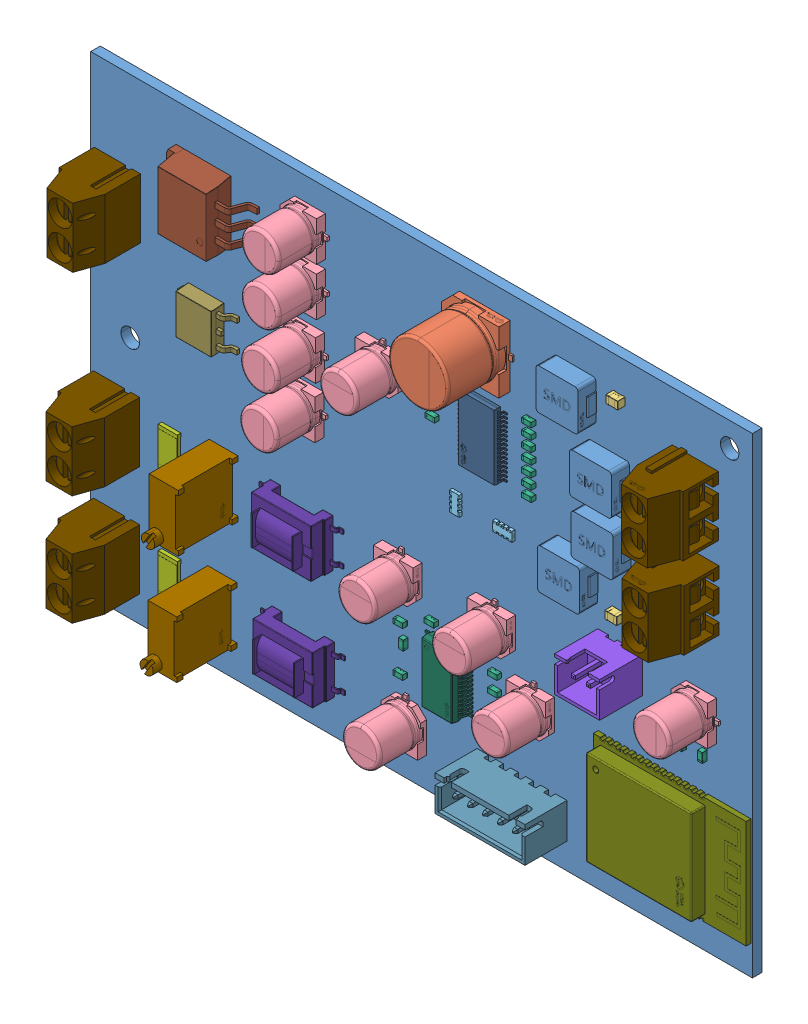
SolidWorks assembly 3D_I2SInputAmp_1_2024-11-02, configuration 默认. Lengths in mm.
Overall size (110.46 78.71 15.8).
191 component instances, 19 part files, 0 mates.
Components (placement in the parent):
- 3D_I2SInputAmp_1_2024-11-02.step-1: 3D_I2SInputAmp_1_2024-11-02.step [默认] at origin size (110.46 78.71 15.8)
  - 2uP9-L2.step-1: 2uP9-L2.step [默认] at (86.2332 60.9601 1.6001) size (7.42 6.8 3.05)
    - IND-SMD_L7.3-W6.8.step-1: IND-SMD_L7.3-W6.8.step [默认] at origin size (7.42 6.8 3.05)
      - SOLID.step-1: SOLID.step [默认] at origin size (7.42 6.8 3.05)
  - 2uP9-L3.step-1: 2uP9-L3.step [默认] at (86.4872 52.1971 1.6001) size (7.42 6.8 3.05)
    - IND-SMD_L7.3-W6.8.step-1: IND-SMD_L7.3-W6.8.step [默认] at origin size (7.42 6.8 3.05)
      - SOLID.step-1: SOLID.step [默认] at origin size (7.42 6.8 3.05)
  - 2uP9-L4.step-1: 2uP9-L4.step [默认] at (80.8992 44.4501 1.6001) size (7.42 6.8 3.05)
    - IND-SMD_L7.3-W6.8.step-1: IND-SMD_L7.3-W6.8.step [默认] at origin size (7.42 6.8 3.05)
      - SOLID.step-1: SOLID.step [默认] at origin size (7.42 6.8 3.05)
  - 2uP9-L1.step-1: 2uP9-L1.step [默认] at (80.6452 70.3581 1.6001) size (7.42 6.8 3.05)
    - IND-SMD_L7.3-W6.8.step-1: IND-SMD_L7.3-W6.8.step [默认] at origin size (7.42 6.8 3.05)
      - SOLID.step-1: SOLID.step [默认] at origin size (7.42 6.8 3.05)
  - 2uP9-C111.step-1: 2uP9-C111.step [默认] at (64.6431 69.7231 1.6001) size (11.6 10.3 10.21)
    - CAP-SMD_BD10.0-L10.3-W10.3-LS11.0-FD.step-1: CAP-SMD_BD10.0-L10.3-W10.3-LS11.0-FD.step [默认] at origin size (11.6 10.3 10.21)
      - COMPOUND.step-1: COMPOUND.step [默认] at origin size (11.6 10.3 10.21)
  - 2uP9-C108.step-1: 2uP9-C108.step [默认] at (87.8528 41.5212 1.6001) x (-1 0 0) z (0 0 1) size (2 1.3 1.3)
    - C0805.step-1: C0805.step [默认] at origin size (2 1.3 1.3)
      - SOLID-0.step-1: SOLID-0.step [默认] at origin size (2 1.3 1.3)
  - 2uP9-C109.step-1: 2uP9-C109.step [默认] at (92.4562 48.6411 1.6001) x (0 1 0) z (0 0 1) size (2 1.3 1.3)
    - C0805.step-1: C0805.step [默认] at origin size (2 1.3 1.3)
      - SOLID-0.step-1: SOLID-0.step [默认] at origin size (2 1.3 1.3)
  - 2uP9-C110.step-1: 2uP9-C110.step [默认] at (93.2182 62.7381 1.6001) x (0 -1 0) z (0 0 1) size (2 1.3 1.3)
    - C0805.step-1: C0805.step [默认] at origin size (2 1.3 1.3)
      - SOLID-0.step-1: SOLID-0.step [默认] at origin size (2 1.3 1.3)
  - 2uP9-C107.step-1: 2uP9-C107.step [默认] at (88.0112 72.7711 1.6001) size (2 1.3 1.3)
    - C0805.step-1: C0805.step [默认] at origin size (2 1.3 1.3)
      - SOLID-0.step-1: SOLID-0.step [默认] at origin size (2 1.3 1.3)
  - 2uP9-C93.step-1: 2uP9-C93.step [默认] at (35.6871 71.6281 1.6001) size (7.8 6.6 7.75)
    - CAP-SMD_BD6.3-L6.6-W6.6-FD.step-1: CAP-SMD_BD6.3-L6.6-W6.6-FD.step [默认] at origin size (7.8 6.6 7.75)
      - SOLID-1.step-1: SOLID-1.step [默认] at origin size (7.8 6.6 7.75)
  - 2uP9-C94.step-1: 2uP9-C94.step [默认] at (35.6871 63.6271 1.6001) size (7.8 6.6 7.75)
    - CAP-SMD_BD6.3-L6.6-W6.6-FD.step-1: CAP-SMD_BD6.3-L6.6-W6.6-FD.step [默认] at origin size (7.8 6.6 7.75)
      - SOLID-1.step-1: SOLID-1.step [默认] at origin size (7.8 6.6 7.75)
  - 2uP9-C112.step-1: 2uP9-C112.step [默认] at (48.7681 57.7851 1.6001) x (0 1 0) z (0 0 1) size (7.8 6.6 7.75)
    - CAP-SMD_BD6.3-L6.6-W6.6-FD.step-1: CAP-SMD_BD6.3-L6.6-W6.6-FD.step [默认] at origin size (7.8 6.6 7.75)
      - SOLID-1.step-1: SOLID-1.step [默认] at origin size (7.8 6.6 7.75)
  - 2uP9-C113.step-1: 2uP9-C113.step [默认] at (35.4331 45.7201 1.6001) size (7.8 6.6 7.75)
    - CAP-SMD_BD6.3-L6.6-W6.6-FD.step-1: CAP-SMD_BD6.3-L6.6-W6.6-FD.step [默认] at origin size (7.8 6.6 7.75)
      - SOLID-1.step-1: SOLID-1.step [默认] at origin size (7.8 6.6 7.75)
  - 2uP9-C114.step-1: 2uP9-C114.step [默认] at (35.5601 54.3561 1.6001) size (7.8 6.6 7.75)
    - CAP-SMD_BD6.3-L6.6-W6.6-FD.step-1: CAP-SMD_BD6.3-L6.6-W6.6-FD.step [默认] at origin size (7.8 6.6 7.75)
      - SOLID-1.step-1: SOLID-1.step [默认] at origin size (7.8 6.6 7.75)
  - 2uP9-C118.step-1: 2uP9-C118.step [默认] at (51.8161 29.2101 1.6001) x (0 1 0) z (0 0 1) size (7.8 6.6 7.75)
    - CAP-SMD_BD6.3-L6.6-W6.6-FD.step-1: CAP-SMD_BD6.3-L6.6-W6.6-FD.step [默认] at origin size (7.8 6.6 7.75)
      - SOLID-1.step-1: SOLID-1.step [默认] at origin size (7.8 6.6 7.75)
  - 2uP9-C120.step-1: 2uP9-C120.step [默认] at (67.4371 29.4641 1.6001) x (0 1 0) z (0 0 1) size (7.8 6.6 7.75)
    - CAP-SMD_BD6.3-L6.6-W6.6-FD.step-1: CAP-SMD_BD6.3-L6.6-W6.6-FD.step [默认] at origin size (7.8 6.6 7.75)
      - SOLID-1.step-1: SOLID-1.step [默认] at origin size (7.8 6.6 7.75)
  - 2uP9-C124.step-1: 2uP9-C124.step [默认] at (52.5781 8.382 1.6001) x (0 -1 0) z (0 0 1) size (7.8 6.6 7.75)
    - CAP-SMD_BD6.3-L6.6-W6.6-FD.step-1: CAP-SMD_BD6.3-L6.6-W6.6-FD.step [默认] at origin size (7.8 6.6 7.75)
      - SOLID-1.step-1: SOLID-1.step [默认] at origin size (7.8 6.6 7.75)
  - 2uP9-C125.step-1: 2uP9-C125.step [默认] at (73.9141 20.828 1.6001) x (0 1 0) z (0 0 1) size (7.8 6.6 7.75)
    - CAP-SMD_BD6.3-L6.6-W6.6-FD.step-1: CAP-SMD_BD6.3-L6.6-W6.6-FD.step [默认] at origin size (7.8 6.6 7.75)
      - SOLID-1.step-1: SOLID-1.step [默认] at origin size (7.8 6.6 7.75)
  - 2uP9-C51.step-1: 2uP9-C51.step [默认] at (100.9845 34.2354 1.6001) size (7.8 6.6 7.75)
    - CAP-SMD_BD6.3-L6.6-W6.6-FD.step-1: CAP-SMD_BD6.3-L6.6-W6.6-FD.step [默认] at origin size (7.8 6.6 7.75)
      - SOLID-1.step-1: SOLID-1.step [默认] at origin size (7.8 6.6 7.75)
  - 2uP9-RN4.step-1: 2uP9-RN4.step [默认] at (60.9601 44.1961 1.6001) x (0 1 0) z (0 0 1) size (3.2 1.6 0.5)
    - RES-ARRAY-SMD_0603-8P-L3.2-W1.6-BL.step-1: RES-ARRAY-SMD_0603-8P-L3.2-W1.6-BL.step [默认] at origin size (3.2 1.6 0.5)
      - COMPOUND-2.step-1: COMPOUND-2.step [默认] at origin size (3.2 1.6 0.5)
  - 2uP9-RN3.step-1: 2uP9-RN3.step [默认] at (68.9611 44.1961 1.6001) size (3.2 1.6 0.5)
    - RES-ARRAY-SMD_0603-8P-L3.2-W1.6-BL.step-1: RES-ARRAY-SMD_0603-8P-L3.2-W1.6-BL.step [默认] at origin size (3.2 1.6 0.5)
      - COMPOUND-2.step-1: COMPOUND-2.step [默认] at origin size (3.2 1.6 0.5)
  - 2uP9-C52.step-1: 2uP9-C52.step [默认] at (98.8255 28.3934 1.6001) x (0 -1 0) z (0 0 1) size (1.6 0.8 0.8)
    - C0603.step-1: C0603.step [默认] at origin size (1.6 0.8 0.8)
      - SOLID-3.step-1: SOLID-3.step [默认] at origin size (1.6 0.8 0.8)
  - 2uP9-C95.step-1: 2uP9-C95.step [默认] at (57.2771 61.0871 1.6001) size (1.6 0.8 0.8)
    - C0603.step-1: C0603.step [默认] at origin size (1.6 0.8 0.8)
      - SOLID-3.step-1: SOLID-3.step [默认] at origin size (1.6 0.8 0.8)
  - 2uP9-C96.step-1: 2uP9-C96.step [默认] at (73.2791 62.2301 1.6001) size (1.6 0.8 0.8)
    - C0603.step-1: C0603.step [默认] at origin size (1.6 0.8 0.8)
      - SOLID-3.step-1: SOLID-3.step [默认] at origin size (1.6 0.8 0.8)
  - 2uP9-C97.step-1: 2uP9-C97.step [默认] at (56.0071 57.9121 1.6001) x (0 1 0) z (0 0 1) size (1.6 0.8 0.8)
    - C0603.step-1: C0603.step [默认] at origin size (1.6 0.8 0.8)
      - SOLID-3.step-1: SOLID-3.step [默认] at origin size (1.6 0.8 0.8)
  - 2uP9-C98.step-1: 2uP9-C98.step [默认] at (57.9121 57.9121 1.6001) x (0 1 0) z (0 0 1) size (1.6 0.8 0.8)
    - C0603.step-1: C0603.step [默认] at origin size (1.6 0.8 0.8)
      - SOLID-3.step-1: SOLID-3.step [默认] at origin size (1.6 0.8 0.8)
  - 2uP9-C99.step-1: 2uP9-C99.step [默认] at (73.2791 60.431 1.6001) x (-1 0 0) z (0 0 1) size (1.6 0.8 0.8)
    - C0603.step-1: C0603.step [默认] at origin size (1.6 0.8 0.8)
      - SOLID-3.step-1: SOLID-3.step [默认] at origin size (1.6 0.8 0.8)
  - 2uP9-C100.step-1: 2uP9-C100.step [默认] at (73.2791 56.8326 1.6001) x (-1 0 0) z (0 0 1) size (1.6 0.8 0.8)
    - C0603.step-1: C0603.step [默认] at origin size (1.6 0.8 0.8)
      - SOLID-3.step-1: SOLID-3.step [默认] at origin size (1.6 0.8 0.8)
  - 2uP9-C101.step-1: 2uP9-C101.step [默认] at (73.2791 54.9911 1.6001) x (-1 0 0) z (0 0 1) size (1.6 0.8 0.8)
    - C0603.step-1: C0603.step [默认] at origin size (1.6 0.8 0.8)
      - SOLID-3.step-1: SOLID-3.step [默认] at origin size (1.6 0.8 0.8)
  - 2uP9-C102.step-1: 2uP9-C102.step [默认] at (73.2791 51.4351 1.6001) x (-1 0 0) z (0 0 1) size (1.6 0.8 0.8)
    - C0603.step-1: C0603.step [默认] at origin size (1.6 0.8 0.8)
      - SOLID-3.step-1: SOLID-3.step [默认] at origin size (1.6 0.8 0.8)
  - 2uP9-C103.step-1: 2uP9-C103.step [默认] at (57.1501 54.8641 1.6001) x (-1 0 0) z (0 0 1) size (1.6 0.8 0.8)
    - C0603.step-1: C0603.step [默认] at origin size (1.6 0.8 0.8)
      - SOLID-3.step-1: SOLID-3.step [默认] at origin size (1.6 0.8 0.8)
  - 2uP9-C104.step-1: 2uP9-C104.step [默认] at (57.2771 63.1191 1.6001) x (-1 0 0) z (0 0 1) size (1.6 0.8 0.8)
    - C0603.step-1: C0603.step [默认] at origin size (1.6 0.8 0.8)
      - SOLID-3.step-1: SOLID-3.step [默认] at origin size (1.6 0.8 0.8)
  - 2uP9-C105.step-1: 2uP9-C105.step [默认] at (73.2637 58.6372 1.6001) x (-1 0 0) z (0 0 1) size (1.6 0.8 0.8)
    - C0603.step-1: C0603.step [默认] at origin size (1.6 0.8 0.8)
      - SOLID-3.step-1: SOLID-3.step [默认] at origin size (1.6 0.8 0.8)
  - 2uP9-C106.step-1: 2uP9-C106.step [默认] at (73.2791 53.2131 1.6001) x (-1 0 0) z (0 0 1) size (1.6 0.8 0.8)
    - C0603.step-1: C0603.step [默认] at origin size (1.6 0.8 0.8)
      - SOLID-3.step-1: SOLID-3.step [默认] at origin size (1.6 0.8 0.8)
  - 2uP9-C115.step-1: 2uP9-C115.step [默认] at (51.8161 14.986 1.6001) size (1.6 0.8 0.8)
    - C0603.step-1: C0603.step [默认] at origin size (1.6 0.8 0.8)
      - SOLID-3.step-1: SOLID-3.step [默认] at origin size (1.6 0.8 0.8)
  - 2uP9-C116.step-1: 2uP9-C116.step [默认] at (67.5641 17.78 1.6001) x (-1 0 0) z (0 0 1) size (1.6 0.8 0.8)
    - C0603.step-1: C0603.step [默认] at origin size (1.6 0.8 0.8)
      - SOLID-3.step-1: SOLID-3.step [默认] at origin size (1.6 0.8 0.8)
  - 2uP9-C117.step-1: 2uP9-C117.step [默认] at (57.0231 25.1461 1.6001) size (1.6 0.8 0.8)
    - C0603.step-1: C0603.step [默认] at origin size (1.6 0.8 0.8)
      - SOLID-3.step-1: SOLID-3.step [默认] at origin size (1.6 0.8 0.8)
  - 2uP9-C119.step-1: 2uP9-C119.step [默认] at (62.3571 25.1461 1.6001) x (-1 0 0) z (0 0 1) size (1.6 0.8 0.8)
    - C0603.step-1: C0603.step [默认] at origin size (1.6 0.8 0.8)
      - SOLID-3.step-1: SOLID-3.step [默认] at origin size (1.6 0.8 0.8)
  - 2uP9-C121.step-1: 2uP9-C121.step [默认] at (51.8161 22.479 1.6001) x (-1 0 0) z (0 0 1) size (1.6 0.8 0.8)
    - C0603.step-1: C0603.step [默认] at origin size (1.6 0.8 0.8)
      - SOLID-3.step-1: SOLID-3.step [默认] at origin size (1.6 0.8 0.8)
  - 2uP9-C123.step-1: 2uP9-C123.step [默认] at (67.5641 22.86 1.6001) size (1.6 0.8 0.8)
    - C0603.step-1: C0603.step [默认] at origin size (1.6 0.8 0.8)
      - SOLID-3.step-1: SOLID-3.step [默认] at origin size (1.6 0.8 0.8)
  - 2uP9-C126.step-1: 2uP9-C126.step [默认] at (67.5641 20.32 1.6001) x (-1 0 0) z (0 0 1) size (1.6 0.8 0.8)
    - C0603.step-1: C0603.step [默认] at origin size (1.6 0.8 0.8)
      - SOLID-3.step-1: SOLID-3.step [默认] at origin size (1.6 0.8 0.8)
  - 2uP9-C127.step-1: 2uP9-C127.step [默认] at (52.3241 19.685 1.6001) x (0 1 0) z (0 0 1) size (1.6 0.8 0.8)
    - C0603.step-1: C0603.step [默认] at origin size (1.6 0.8 0.8)
      - SOLID-3.step-1: SOLID-3.step [默认] at origin size (1.6 0.8 0.8)
  - 2uP9-C50.step-1: 2uP9-C50.step [默认] at (102.2545 28.3934 1.6001) x (0 1 0) z (0 0 1) size (1.6 0.8 0.8)
    - C0603.step-1: C0603.step [默认] at origin size (1.6 0.8 0.8)
      - SOLID-3.step-1: SOLID-3.step [默认] at origin size (1.6 0.8 0.8)
  - 2uP9-R29.step-1: 2uP9-R29.step [默认] at (13.208 9.652 1.6001) x (0 1 0) z (0 0 1) size (6.3 3.2 0.61)
    - R2512.step-1: R2512.step [默认] at origin size (6.3 3.2 0.61)
      - COMPOUND-4.step-1: COMPOUND-4.step [默认] at origin size (6.3 3.2 0.61)
  - 2uP9-R28.step-1: 2uP9-R28.step [默认] at (13.208 27.9401 1.6001) x (0 1 0) z (0 0 1) size (6.3 3.2 0.61)
    - R2512.step-1: R2512.step [默认] at origin size (6.3 3.2 0.61)
      - COMPOUND-4.step-1: COMPOUND-4.step [默认] at origin size (6.3 3.2 0.61)
  - 2uP9-SETTING0.step-1: 2uP9-SETTING0.step [默认] at (88.2652 35.3061 1.6001) size (7.5 5.9 10.6)
    - CONN-TH_2P-P2.50_HX25003-2A.step-1: CONN-TH_2P-P2.50_HX25003-2A.step [默认] at origin size (7.5 5.9 10.6)
      - COMPOUND-5.step-1: COMPOUND-5.step [默认] at origin size (7.5 5.9 10.6)
  - 2uP9-R35.step-1: 2uP9-R35.step [默认] at (21.7482 9.4159 1.6001) x (-1 0 0) z (0 0 1) size (4.85 9.5 15)
    - RES-ADJ-TH_3P-L10.0-W10.0-P2.50-BL-BS.step-1: RES-ADJ-TH_3P-L10.0-W10.0-P2.50-BL-BS.step [默认] at origin size (4.85 9.5 15)
      - SOLID-6.step-1: SOLID-6.step [默认] at origin size (4.85 9.5 15)
  - 2uP9-R34.step-1: 2uP9-R34.step [默认] at (21.971 27.8131 1.6001) x (-1 0 0) z (0 0 1) size (4.85 9.5 15)
    - RES-ADJ-TH_3P-L10.0-W10.0-P2.50-BL-BS.step-1: RES-ADJ-TH_3P-L10.0-W10.0-P2.50-BL-BS.step [默认] at origin size (4.85 9.5 15)
      - SOLID-6.step-1: SOLID-6.step [默认] at origin size (4.85 9.5 15)
  - 2uP9-U15.step-1: 2uP9-U15.step [默认] at (65.2781 56.2611 1.6001) x (0 -1 0) z (0 0 1) size (11 8.1 1.16)
    - HTSSOP-32_L11.0-W6.1-P0.65-LS8.1-BL-EP-4.step-1: HTSSOP-32_L11.0-W6.1-P0.65-LS8.1-BL-EP-4.step [默认] at origin size (11 8.1 1.16)
      - SOLID-7.step-1: SOLID-7.step [默认] at origin size (11 8.1 1.16)
  - 2uP9-U20.step-1: 2uP9-U20.step [默认] at (22.535 67.3391 1.6001) size (14.23 10.2 4.5)
    - TO-263-3_L8.6-W10.2-P2.54-LS14.4-BR.step-1: TO-263-3_L8.6-W10.2-P2.54-LS14.4-BR.step [默认] at origin size (14.23 10.2 4.5)
      - COMPOUND-8.step-1: COMPOUND-8.step [默认] at origin size (14.23 10.2 4.5)
  - 2uP9-U23.step-1: 2uP9-U23.step [默认] at (20.701 50.1651 1.6001) size (9.92 6.6 2.3)
    - TO-252-2_L6.6-W6.1-P4.57-LS9.9-BR-CW.step-1: TO-252-2_L6.6-W6.1-P4.57-LS9.9-BR-CW.step [默认] at origin size (9.92 6.6 2.3)
      - COMPOUND-9.step-1: COMPOUND-9.step [默认] at origin size (9.92 6.6 2.3)
  - 2uP9-R33.step-1: 2uP9-R33.step [默认] at (96.2855 28.3934 1.6001) x (0 1 0) z (0 0 1) size (1.62 0.81 0.45)
    - R0603.step-1: R0603.step [默认] at origin size (1.62 0.81 0.45)
      - COMPOUND-10.step-1: COMPOUND-10.step [默认] at origin size (1.62 0.81 0.45)
  - 2uP9-R32.step-1: 2uP9-R32.step [默认] at (92.7295 28.5204 1.6001) x (0 1 0) z (0 0 1) size (1.62 0.81 0.45)
    - R0603.step-1: R0603.step [默认] at origin size (1.62 0.81 0.45)
      - COMPOUND-10.step-1: COMPOUND-10.step [默认] at origin size (1.62 0.81 0.45)
  - 2uP9-U14.step-1: 2uP9-U14.step [默认] at (71.7551 7.62 1.6001) x (-1 0 0) z (0 0 1) size (15 5.91 10.4)
    - CONN-TH_5P-P2.50_ZX-XH2.54-5PZZ.step-1: CONN-TH_5P-P2.50_ZX-XH2.54-5PZZ.step [默认] at origin size (15 5.91 10.4)
      - SOLID-11.step-1: SOLID-11.step [默认] at origin size (15 5.91 10.4)
  - 2uP9-U16.step-1: 2uP9-U16.step [默认] at (59.6901 18.796 1.6001) x (0 -1 0) z (0 0 1) size (10.2 7.8 2.2)
    - SSOP-28_L10.2-W5.3-P0.65-LS7.8-BL.step-1: SSOP-28_L10.2-W5.3-P0.65-LS7.8-BL.step [默认] at origin size (10.2 7.8 2.2)
      - SOLID-12.step-1: SOLID-12.step [默认] at origin size (10.2 7.8 2.2)
  - 2uP9-U1.step-1: 2uP9-U1.step [默认] at (93.4915 13.9153 1.6001) x (0 -1 0) z (0 0 1) size (18 25.5 3.12)
    - WIFIM-SMD_ESP32-WROOM-32-N4.step-1: WIFIM-SMD_ESP32-WROOM-32-N4.step [默认] at origin size (18 25.5 3.12)
      - SOLID-13.step-1: SOLID-13.step [默认] at origin size (18 25.5 3.12)
  - 2uP9-U19.step-1: 2uP9-U19.step [默认] at (35.3061 9.779 1.6001) x (0 -1 0) z (0 0 1) size (8.01 14 5.02)
    - XFMR-SMD_L10.5-W8.0-P5.00-LS14.0_ED8-600.step-1: XFMR-SMD_L10.5-W8.0-P5.00-LS14.0_ED8-600.step [默认] at origin size (8.01 14 5.02)
      - COMPOUND-14.step-1: COMPOUND-14.step [默认] at origin size (8.01 14 5.02)
  - 2uP9-U18.step-1: 2uP9-U18.step [默认] at (35.0521 27.9401 1.6001) x (0 -1 0) z (0 0 1) size (8.01 14 5.02)
    - XFMR-SMD_L10.5-W8.0-P5.00-LS14.0_ED8-600.step-1: XFMR-SMD_L10.5-W8.0-P5.00-LS14.0_ED8-600.step [默认] at origin size (8.01 14 5.02)
      - COMPOUND-14.step-1: COMPOUND-14.step [默认] at origin size (8.01 14 5.02)
  - 2uP9-U12.step-1: 2uP9-U12.step [默认] at (3.937 27.8131 1.6001) x (0 -1 0) z (0 0 1) size (10.4 7.7 14.2)
    - CONN-TH_P5.00_KF301-5.0-2P.step-1: CONN-TH_P5.00_KF301-5.0-2P.step [默认] at origin size (10.4 7.7 14.2)
      - COMPOUND-15.step-1: COMPOUND-15.step [默认] at origin size (10.4 7.7 14.2)
  - 2uP9-U13.step-1: 2uP9-U13.step [默认] at (3.937 9.398 1.6001) x (0 -1 0) z (0 0 1) size (10.4 7.7 14.2)
    - CONN-TH_P5.00_KF301-5.0-2P.step-1: CONN-TH_P5.00_KF301-5.0-2P.step [默认] at origin size (10.4 7.7 14.2)
      - COMPOUND-15.step-1: COMPOUND-15.step [默认] at origin size (10.4 7.7 14.2)
  - 2uP9-U21.step-1: 2uP9-U21.step [默认] at (100.8382 65.4051 1.6001) x (0 1 0) z (0 0 1) size (10.4 7.7 14.2)
    - CONN-TH_P5.00_KF301-5.0-2P.step-1: CONN-TH_P5.00_KF301-5.0-2P.step [默认] at origin size (10.4 7.7 14.2)
      - COMPOUND-15.step-1: COMPOUND-15.step [默认] at origin size (10.4 7.7 14.2)
  - 2uP9-U22.step-1: 2uP9-U22.step [默认] at (100.9652 51.8161 1.6001) x (0 1 0) z (0 0 1) size (10.4 7.7 14.2)
    - CONN-TH_P5.00_KF301-5.0-2P.step-1: CONN-TH_P5.00_KF301-5.0-2P.step [默认] at origin size (10.4 7.7 14.2)
      - COMPOUND-15.step-1: COMPOUND-15.step [默认] at origin size (10.4 7.7 14.2)
  - 2uP9-U9.step-1: 2uP9-U9.step [默认] at (4.064 60.1981 1.6001) x (0 -1 0) z (0 0 1) size (10.4 7.7 14.2)
    - CONN-TH_P5.00_KF301-5.0-2P.step-1: CONN-TH_P5.00_KF301-5.0-2P.step [默认] at origin size (10.4 7.7 14.2)
      - COMPOUND-15.step-1: COMPOUND-15.step [默认] at origin size (10.4 7.7 14.2)
  - Board.step-1: Board.step [默认] at origin size (110.46 78.71 1.6)
